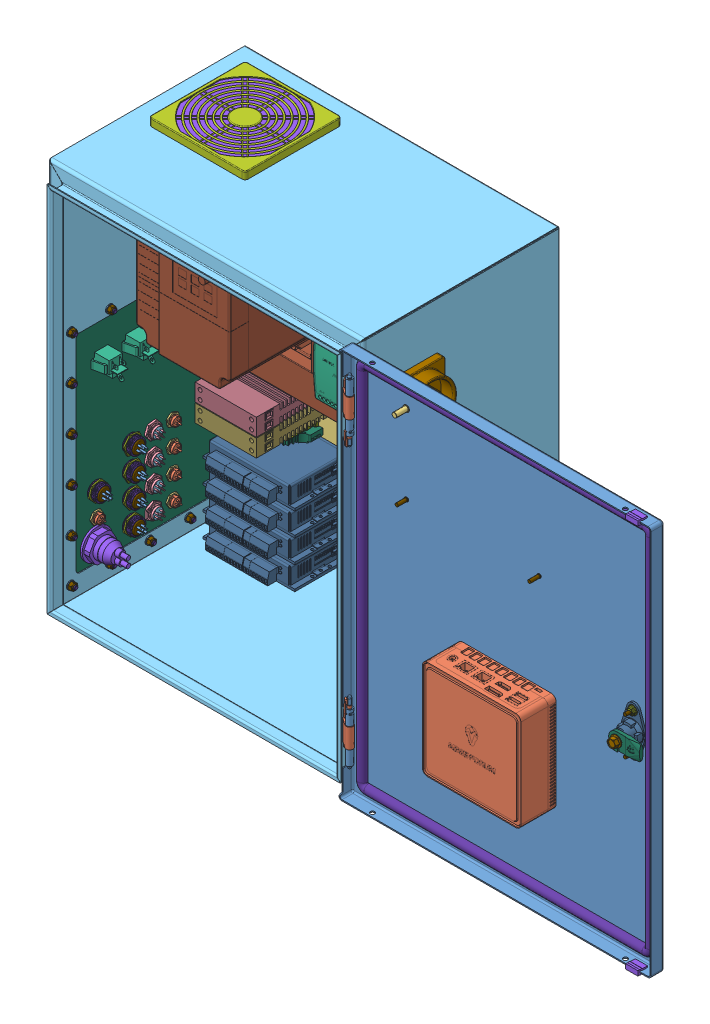
SolidWorks assembly CNC Control Panel, configuration Door Open. Lengths in mm.
Overall size (839.73 526.05 313.88).
272 component instances, 67 part files, 147 mates.
Components (placement in the parent):
- YuCo YC-20X16X10-UL-1: YuCo YC-20X16X10-UL [Door Open] x (-1 0 0) z (0 0 1) size (799.63 509.27 290.8)
  - 87929507-1: 87929507 [Default] at (-197.7898 -139.7 266.2428) x (0 -1 0) z (-0.965926 0 0.258819) size (80.01 7.68 4.83)
    - 87929767-1: 87929767 [Default] at origin size (80.01 4.75 4.75)
    - 87929769_Installed on Pin-1: 87929769_Installed on Pin [Default] at (1.778 3.6068 0) size (17.91 7.45 4.83)
  - 87934540-1: 87934540 [Default] at origin size (406.4 508 269.11)
    - 99401225-1: 99401225 [Default] at (-202.0316 -214.7316 214.7316) x (0 -1 0) z (0 0 1) size (8 16 8)
    - 23271001_After Weld-1: 23271001_After Weld [Default] at (-167.2336 -218.0336 1.1684) x (1 0 0) z (0 -1 0) size (15.88 38.1 15.88)
    - 23271001_After Weld-2: 23271001_After Weld [Default] at (-167.2336 218.0336 1.1684) x (1 0 0) z (0 -1 0) size (15.88 38.1 15.88)
    - 23271001_After Weld-3: 23271001_After Weld [Default] at (167.2336 -218.0336 1.1684) x (1 0 0) z (0 -1 0) size (15.88 38.1 15.88)
    - 23271001_After Weld-4: 23271001_After Weld [Default] at (167.2336 218.0336 1.1684) x (-1 0 0) z (0 1 0) size (15.88 38.1 15.88)
    - 87934343_default-1: 87934343_default [Default] at origin size (406.4 508 269.11)
  - 89076399-1: 89076399 [Default] at (-185.1152 184.15 251.2568) x (0 1 0) z (-1 0 0) size (53.98 24.05 15.83)
    - 89076193-1: 89076193 [Default] at origin size (53.98 23 15.83)
    - 89056623-1: 89056623 [Default] at (0 0 7.112) x (-1 0 0) z (0 -1 0) size (49.12 14 1.57)
  - 89076399-2: 89076399 [Default] at (-185.1152 -184.15 251.2568) x (0 1 0) z (-1 0 0) size (53.98 24.05 15.83)
    - 89076193-1: 89076193 [Default] at origin size (53.98 23 15.83)
    - 89056623-1: 89056623 [Default] at (0 0 7.112) x (-1 0 0) z (0 -1 0) size (49.12 14 1.57)
  - 87937923_assy-1: 87937923_assy [Default] at (-395.0843 0 260.0452) x (-1 0 0) z (0 0 -1) size (402.69 509.27 33.01)
    - 64138001-1: 64138001 [Default] at (179.1589 250.7528 -18.99) x (0 0.043619 0.999048) z (1 0 0) size (12.45 6.6 15.75)
    - 64101001-1: 64101001 [Default] at (163.7162 2.0815 -11.0121) size (45.67 63.4 33.01)
      - 87927840_87927840-1: 87927840_87927840 [Default] at (0.5837 -2.0815 -13.7669) x (0 -1 0) z (0 0 -1) size (14 14 15.97)
      - 64201001-1: 64201001 [Default] at (0.5837 -2.0815 11.0121) size (30.48 63.4 19.81)
      - 87541994_Installed Height-1: 87541994_Installed Height [Default] at (0.5837 -2.0815 -0.4393) x (0 -1 0) z (-1 0 0) size (15.37 3.57 15.57)
      - 87541995-1: 87541995 [Default] at (0.5837 -2.0815 0.0901) size (16.26 16.26 1.78)
      - 64210001-1: 64210001 [Default] at (0.5837 -2.0815 8.7261) size (26.42 26.42 4.55)
      - 64202001-1: 64202001 [Default] at (-17.6801 -2.0815 2.3184) x (1 0 0) z (0 -1 0) size (15.88 25.4 15.88)
      - 64203001-1: 64203001 [Default] at (-128.4369 7.7022 -12.7369) size (40.59 20.36 8)
    - 64138001-2: 64138001 [Default] at (179.1589 -251.3798 -18.99) x (0 0.043619 0.999048) z (1 0 0) size (12.45 6.6 15.75)
    - 87932903-1: 87932903 [Default] at (164.2999 23.8125 -6.4503) x (0 -1 0) z (1 0 0) size (11.43 5.65 11.43)
    - 87932903-2: 87932903 [Default] at (164.2999 -23.8125 -6.4503) x (0 -1 0) z (1 0 0) size (11.43 5.65 11.43)
    - 89057561-1: 89057561 [Default] at (-185.8264 0 0) x (1 0 0) z (0 1 0) size (385.34 6.35 486.94)
    - 87937963_weldment-1: 87937963_weldment [Default] at origin size (402.69 503.96 17.74)
      - 87931362_87931362-1: 87931362_87931362 [Default] at (164.2999 23.8125 0) x (-1 0 0) z (0 -1 0) size (5 13.61 5)
      - 87931362_87931362-2: 87931362_87931362 [Default] at (-129.8829 -110.6678 0) x (1 0 0) z (0 1 0) size (5 13.61 5)
      - 87931362_87931362-3: 87931362_87931362 [Default] at (41.0591 -110.6678 0) x (1 0 0) z (0 1 0) size (5 13.61 5)
      - 87937909-1: 87937909 [Default] at origin size (402.69 503.96 17.74)
      - 99401225-1: 99401225 [Default] at (-129.8829 -212.2678 0) x (1 0 0) z (0 1 0) size (8 16 8)
      - 87931362_87931362-4: 87931362_87931362 [Default] at (164.2999 -23.8125 0) x (-1 0 0) z (0 -1 0) size (5 13.61 5)
  - 87543027-1: 87543027 [Default] at (-198.0692 -184.15 254) x (0 -1 0) z (-1 0 0) size (52.83 16.6 16.78)
  - 87929507-2: 87929507 [Default] at (-197.7898 139.7 266.2428) x (0 1 0) z (0.965926 0 -0.258819) size (80.01 7.68 4.83)
    - 87929767-1: 87929767 [Default] at origin size (80.01 4.75 4.75)
    - 87929769_Installed on Pin-1: 87929769_Installed on Pin [Default] at (1.778 3.6068 0) size (17.91 7.45 4.83)
  - 87543027-2: 87543027 [Default] at (-198.0692 184.15 254) x (0 -1 0) z (-1 0 0) size (52.83 16.6 16.78)
  - 64403004-1: 64403004 [Default] at (0 0 23.5204) size (360.68 462.28 2.46)
- SCN-1000-48-1: SCN-1000-48 [Default] at (102.34 60.64 91.9842) x (0 -1 0) z (0 0 1) size (331 68 132)
  - SCN-1000-48 PSU-1: SCN-1000-48 PSU [Default] at origin size (331 68 132)
  - 19155K930_EQUIPMENT COOLING FAN ACCESSORY-1: 19155K930_EQUIPMENT COOLING FAN ACCESSORY [19155K93] at (145.5 34 -35) x (0 -1 0) z (0 0 1) size (57.8 4.4 57.8)
- ALIM MEAN WELL MDR-1: ALIM MEAN WELL MDR [MDR-60-24] at (75.44 73.64 129.4842) x (-1 0 0) z (0 0 1) size (40 90 100.01)
- ALIM MEAN WELL MDR-2: ALIM MEAN WELL MDR [MDR-60-5] at (33.44 73.64 129.4842) x (-1 0 0) z (0 0 1) size (40 90 100.01)
- AXBB-E-1: AXBB-E [Default] at (38.135 -161.215 36.9842) x (-1 0 0) z (0 1 0) size (97.39 26.5 120)
- UCSB-1: UCSB [Default] at (25.6757 -62.365 38.4842) x (-1 0 0) z (0 1 0) size (116.46 15.11 67.7)
- CNCDrive_Parts_Mount-1: CNCDrive_Parts_Mount [Default] at (38.135 -161.215 28.9842) size (93.95 191.55 11)
- CL57Y Stepper Driver-1: CL57Y Stepper Driver [Default] at (-96.34 -223.14 63.8842) x (0 0 1) z (0 1 0) size (89.31 118 24.2)
- 7578K262_SLOTTED WIRE DUCT WITH SNAP-ON COVER-1: 7578K262_SLOTTED WIRE DUCT WITH SNAP-ON COVER [4in] at (-12.0928 118.3376 25.9842) x (-1 0 0) z (0 1 0) size (39.88 59.94 101.6)
- 8961K150_DIN RAIL (1)-1: 8961K150_DIN RAIL (1) [3.5in] at (510.44 73.64 25.9842) x (0 0 1) z (-1 0 0) size (7.5 35 88.9)
- 7578K262_SLOTTED WIRE DUCT WITH SNAP-ON COVER-3: 7578K262_SLOTTED WIRE DUCT WITH SNAP-ON COVER [10in] at (-158.56 -3.2012 25.9842) x (0 -1 0) z (-1 0 0) size (39.88 59.94 254.14)
- 8961K150_DIN RAIL (1)-2: 8961K150_DIN RAIL (1) [3in] at (-102.84 395.86 25.9842) x (0 0 1) z (0 -1 0) size (7.5 35 76.2)
- 8961K150_DIN RAIL (1)-3: 8961K150_DIN RAIL (1) [5in] at (468.34 183.64 25.9842) x (0 0 1) z (-1 0 0) size (7.5 35 127)
- Lovato Electric FB01F1P-4: Lovato Electric FB01F1P [Default] at (-30.16 183.5289 27.4842) size (17.5 88.8 63.77)
- Lovato Electric FB01F1P-5: Lovato Electric FB01F1P [Default] at (-12.16 183.5289 27.4842) size (17.5 88.8 63.77)
- 7641K526_MODULAR DIN RAIL-MOUNT TERMINAL BLOCK-2: 7641K526_MODULAR DIN RAIL-MOUNT TERMINAL BLOCK [7641K526] at (9.84 186.09 73.9842) x (1 0 0) z (0 -1 0) size (8.38 46.95 44.65)
- 7641K350_MODULAR DIN RAIL-MOUNT TERMINAL BLOCK-1: 7641K350_MODULAR DIN RAIL-MOUNT TERMINAL BLOCK [Default] at (92.64 183.44 27.0092) x (1 0 0) z (0 -1 0) size (10.03 34.98 53.45)
- 7641K924_MODULAR DIN RAIL-MOUNT TERMINAL BLOCK-1: 7641K924_MODULAR DIN RAIL-MOUNT TERMINAL BLOCK [7641K924] at (-105.067 -81.644 73.9842) x (0 1 0) z (1 0 0) size (7 46.95 44.65)
- 7641K350_MODULAR DIN RAIL-MOUNT TERMINAL BLOCK-2: 7641K350_MODULAR DIN RAIL-MOUNT TERMINAL BLOCK [Default] at (-102.64 -101.944 27.0092) x (0 -1 0) z (-1 0 0) size (10.03 34.98 53.45)
- M5 Bolt Nut Washer Assembly-1: M5 Bolt Nut Washer Assembly [Default] at (127.6278 68.7129 256.9715) size (14.92 12.73 12.73) (flexible)
  - Trimcraft M5 BSC-1: Trimcraft M5 BSC [5mm x 12mm SST BSC] at (-336.6778 -21.2987 -233.3857) x (0 0 1) z (-1 0 0) size (9.5 9.5 14.92)
  - Trimcraft M5 Nylock Nut-1: Trimcraft M5 Nylock Nut [M5 Nylock Nut] at (-328.5594 -21.2987 -233.3857) x (0 0 1) z (0 1 0) size (8 5.15 9.24)
  - Trimcraft M5 Washer-1: Trimcraft M5 Washer [M5 Flat Washer] at (-328.5594 -21.2987 -233.3857) x (0 0.07132 0.997453) z (-1 0 0) size (10 10 1.1)
  - Trimcraft M5 Washer-2: Trimcraft M5 Washer [M5 Flat Washer] at (-332.8278 -21.2987 -233.3857) x (0 -0.944717 -0.327887) z (-1 0 0) size (10 10 1.1)
- M5 Bolt Nut Washer Assembly-2: M5 Bolt Nut Washer Assembly [Default] at (129.63 85.8442 76.3307) x (0.969846 0.17101 -0.173648) z (0.198566 -0.141314 0.969846) size (17.7 13.8 13.81) (flexible)
  - Trimcraft M5 BSC-1: Trimcraft M5 BSC [5mm x 12mm SST BSC] at (-334.5346 10.5606 -64.1628) x (-0.198566 0.014245 0.979984) z (-0.969846 0.141314 -0.198566) size (9.5 9.5 14.92)
  - Trimcraft M5 Nylock Nut-1: Trimcraft M5 Nylock Nut [M5 Nylock Nut] at (-326.661 9.4134 -62.5507) x (-0.198566 0.014245 0.979984) z (0.141314 0.989862 0.014245) size (8 5.15 9.24)
  - Trimcraft M5 Washer-1: Trimcraft M5 Washer [M5 Flat Washer] at (-326.661 9.4134 -62.5507) x (-0.187981 0.084806 0.978504) z (-0.969846 0.141314 -0.198566) size (10 10 1.1)
  - Trimcraft M5 Washer-2: Trimcraft M5 Washer [M5 Flat Washer] at (-330.8007 10.0166 -63.3983) x (-0.223661 -0.839732 0.494799) z (-0.969846 0.141314 -0.198566) size (10 10 1.1)
- M5 Bolt Nut Washer Assembly-3: M5 Bolt Nut Washer Assembly [Default] at (129.3262 128.9032 16.2035) x (0.883022 0.321394 -0.34202) z (0.418989 -0.211471 0.883022) size (19.17 14.18 15.7) (flexible)
  - Trimcraft M5 BSC-1: Trimcraft M5 BSC [5mm x 12mm SST BSC] at (-362.0061 31.847 -28.5976) x (-0.418989 0.047054 0.906771) z (-0.883022 0.211471 -0.418989) size (9.5 9.5 14.92)
  - Trimcraft M5 Nylock Nut-1: Trimcraft M5 Nylock Nut [M5 Nylock Nut] at (-354.8374 30.1302 -25.1961) x (-0.418989 0.047054 0.906771) z (0.211471 0.976251 0.047054) size (8 5.15 9.24)
  - Trimcraft M5 Washer-1: Trimcraft M5 Washer [M5 Flat Washer] at (-354.8374 30.1302 -25.1961) x (-0.40284 0.116561 0.907818) z (-0.883022 0.211471 -0.418989) size (10 10 1.1)
  - Trimcraft M5 Washer-2: Trimcraft M5 Washer [M5 Flat Washer] at (-358.6065 31.0329 -26.9845) x (-0.397734 -0.81111 0.428846) z (-0.883022 0.211471 -0.418989) size (10 10 1.1)
- M5 Bolt Nut Washer Assembly-4: M5 Bolt Nut Washer Assembly [Default] at (112.6468 166.765 -45.5219) x (0.75 0.433013 -0.5) z (0.625 -0.216506 0.75) size (19.19 14.4 17.44) (flexible)
  - Trimcraft M5 BSC-1: Trimcraft M5 BSC [5mm x 12mm SST BSC] at (-403.4603 61.6518 -9.2057) x (-0.625 0.077324 0.776786) z (-0.75 0.216506 -0.625) size (9.5 9.5 14.92)
  - Trimcraft M5 Nylock Nut-1: Trimcraft M5 Nylock Nut [M5 Nylock Nut] at (-397.3715 59.8941 -4.1317) x (-0.625 0.077324 0.776786) z (0.216506 0.973214 0.077324) size (8 5.15 9.24)
  - Trimcraft M5 Washer-1: Trimcraft M5 Washer [M5 Flat Washer] at (-397.3715 59.8941 -4.1317) x (-0.607967 0.146537 0.780322) z (-0.75 0.216506 -0.625) size (10 10 1.1)
  - Trimcraft M5 Washer-2: Trimcraft M5 Washer [M5 Flat Washer] at (-400.5728 60.8182 -6.7994) x (-0.508622 -0.792851 0.335694) z (-0.75 0.216506 -0.625) size (10 10 1.1)
- M5 Bolt Nut Washer Assembly-5: M5 Bolt Nut Washer Assembly [Default] at (81.8817 192.9931 -105.544) x (0.586824 0.492404 -0.642788) z (0.790379 -0.175893 0.586824) size (17.94 14.06 18.39) (flexible)
  - Trimcraft M5 BSC-1: Trimcraft M5 BSC [5mm x 12mm SST BSC] at (-455.788 90.5376 -9.5391) x (-0.790379 0.08761 0.606321) z (-0.586824 0.175893 -0.790379) size (9.5 9.5 14.92)
  - Trimcraft M5 Nylock Nut-1: Trimcraft M5 Nylock Nut [M5 Nylock Nut] at (-451.0239 89.1096 -3.1224) x (-0.790379 0.08761 0.606321) z (0.175893 0.980503 0.08761) size (8 5.15 9.24)
  - Trimcraft M5 Washer-1: Trimcraft M5 Washer [M5 Flat Washer] at (-451.0239 89.1096 -3.1224) x (-0.775822 0.157317 0.611025) z (-0.586824 0.175893 -0.790379) size (10 10 1.1)
  - Trimcraft M5 Washer-2: Trimcraft M5 Washer [M5 Flat Washer] at (-453.5287 89.8604 -6.4961) x (-0.559424 -0.793767 0.238702) z (-0.586824 0.175893 -0.790379) size (10 10 1.1)
- M5 Bolt Nut Washer Assembly-6: M5 Bolt Nut Washer Assembly [Default] at (42.0554 202.5261 -160.3334) x (0.413176 0.492404 -0.766044) z (0.903335 -0.115201 0.413176) size (16.19 13.98 18.19) (flexible)
  - Trimcraft M5 BSC-1: Trimcraft M5 BSC [5mm x 12mm SST BSC] at (-504.5231 37.339 -42.4506) x (-0.903335 0.073639 0.422567) z (-0.413176 0.115201 -0.903335) size (9.5 9.5 14.92)
  - Trimcraft M5 Nylock Nut-1: Trimcraft M5 Nylock Nut [M5 Nylock Nut] at (-501.1687 36.4037 -35.1169) x (-0.903335 0.073639 0.422567) z (0.115201 0.990609 0.073639) size (8 5.15 9.24)
  - Trimcraft M5 Washer-1: Trimcraft M5 Washer [M5 Flat Washer] at (-501.1687 36.4037 -35.1169) x (-0.892819 0.144102 0.426743) z (-0.413176 0.115201 -0.903335) size (10 10 1.1)
  - Trimcraft M5 Washer-2: Trimcraft M5 Washer [M5 Flat Washer] at (-502.9323 36.8955 -38.9727) x (-0.565922 -0.809644 0.155594) z (-0.413176 0.115201 -0.903335) size (10 10 1.1)
- M5 Bolt Nut Washer Assembly-7: M5 Bolt Nut Washer Assembly [Default] at (0.1494 192.8274 -206.4354) x (0.25 0.433013 -0.866025) z (0.966506 -0.058013 0.25) size (14.6 13.91 17.25) (flexible)
  - Trimcraft M5 BSC-1: Trimcraft M5 BSC [5mm x 12mm SST BSC] at (-539.5682 -32.6411 -78.8416) x (-0.966506 0.044856 0.252692) z (-0.25 0.058013 -0.966506) size (9.5 9.5 14.92)
  - Trimcraft M5 Nylock Nut-1: Trimcraft M5 Nylock Nut [M5 Nylock Nut] at (-537.5386 -33.1121 -70.9951) x (-0.966506 0.044856 0.252692) z (0.058013 0.997308 0.044856) size (8 5.15 9.24)
  - Trimcraft M5 Washer-1: Trimcraft M5 Washer [M5 Flat Washer] at (-537.5386 -33.1121 -70.9951) x (-0.959908 0.11587 0.255248) z (-0.25 0.058013 -0.966506) size (10 10 1.1)
  - Trimcraft M5 Washer-2: Trimcraft M5 Washer [M5 Flat Washer] at (-538.6057 -32.8644 -75.1206) x (-0.549663 -0.830267 0.092343) z (-0.25 0.058013 -0.966506) size (10 10 1.1)
- M5 Bolt Nut Washer Assembly-8: M5 Bolt Nut Washer Assembly [Default] at (-36.1524 164.5811 -240.7794) x (0.116978 0.321394 -0.939693) z (0.992945 -0.019382 0.116978) size (13.83 13.81 16.1) (flexible)
  - Trimcraft M5 BSC-1: Trimcraft M5 BSC [5mm x 12mm SST BSC] at (-552.028 -118.0059 -111.3957) x (-0.992945 0.01723 0.117314) z (-0.116978 0.019382 -0.992945) size (9.5 9.5 14.92)
  - Trimcraft M5 Nylock Nut-1: Trimcraft M5 Nylock Nut [M5 Nylock Nut] at (-551.0783 -118.1633 -103.3346) x (-0.992945 0.01723 0.117314) z (0.019382 0.999664 0.01723) size (8 5.15 9.24)
  - Trimcraft M5 Washer-1: Trimcraft M5 Washer [M5 Flat Washer] at (-551.0783 -118.1633 -103.3346) x (-0.989034 0.088483 0.118244) z (-0.116978 0.019382 -0.992945) size (10 10 1.1)
  - Trimcraft M5 Washer-2: Trimcraft M5 Washer [M5 Flat Washer] at (-551.5776 -118.0806 -107.5729) x (-0.530282 -0.846575 0.045947) z (-0.116978 0.019382 -0.992945) size (10 10 1.1)
- M5 Bolt Nut Washer Assembly-9: M5 Bolt Nut Washer Assembly [Default] at (-59.9382 121.7476 -260.9631) x (0.030154 0.17101 -0.984808) z (0.999542 -0.002598 0.030154) size (13.77 13.74 15.23) (flexible)
  - Trimcraft M5 BSC-1: Trimcraft M5 BSC [5mm x 12mm SST BSC] at (-536.5111 -212.6794 -133.5477) x (-0.999542 0.002521 0.03016) z (-0.030154 0.002598 -0.999542) size (9.5 9.5 14.92)
  - Trimcraft M5 Nylock Nut-1: Trimcraft M5 Nylock Nut [M5 Nylock Nut] at (-536.2663 -212.7005 -125.433) x (-0.999542 0.002521 0.03016) z (0.002598 0.999993 0.002521) size (8 5.15 9.24)
  - Trimcraft M5 Washer-1: Trimcraft M5 Washer [M5 Flat Washer] at (-536.2663 -212.7005 -125.433) x (-0.996811 0.073834 0.030263) z (-0.030154 0.002598 -0.999542) size (10 10 1.1)
  - Trimcraft M5 Washer-2: Trimcraft M5 Washer [M5 Flat Washer] at (-536.395 -212.6894 -129.6995) x (-0.519331 -0.854467 0.013446) z (-0.030154 0.002598 -0.999542) size (10 10 1.1)
- M5 Bolt Nut Washer Assembly-10: M5 Bolt Nut Washer Assembly [Default] at (-66.4389 70.9384 -265.4779) x (0 0 -1) z (1 0 0) size (13.73 13.73 14.92) (flexible)
  - Trimcraft M5 BSC-1: Trimcraft M5 BSC [5mm x 12mm SST BSC] at (-491.8922 -306.3526 -142.6111) x (-1 0 0) z (0 0 -1) size (9.5 9.5 14.92)
  - Trimcraft M5 Nylock Nut-1: Trimcraft M5 Nylock Nut [M5 Nylock Nut] at (-491.8922 -306.3526 -134.4927) x (-1 0 0) z (0 1 0) size (8 5.15 9.24)
  - Trimcraft M5 Washer-1: Trimcraft M5 Washer [M5 Flat Washer] at (-491.8922 -306.3526 -134.4927) x (-0.997453 0.07132 0) z (0 0 -1) size (10 10 1.1)
  - Trimcraft M5 Washer-2: Trimcraft M5 Washer [M5 Flat Washer] at (-491.8922 -306.3526 -138.7611) x (-0.517345 -0.855777 0) z (0 0 -1) size (10 10 1.1)
- M5 Bolt Nut Washer Assembly-11: M5 Bolt Nut Washer Assembly [Default] at (-53.9864 20.2276 -253.8526) x (0.030154 -0.17101 -0.984808) z (0.999542 0.002598 0.030154) size (13.75 13.73 15.23) (flexible)
  - Trimcraft M5 BSC-1: Trimcraft M5 BSC [5mm x 12mm SST BSC] at (-384.1804 -326.3643 -142.6966) x (-0.999542 -0.002521 0.03016) z (-0.030154 -0.002598 -0.999542) size (9.5 9.5 14.92)
  - Trimcraft M5 Nylock Nut-1: Trimcraft M5 Nylock Nut [M5 Nylock Nut] at (-383.9356 -326.3432 -134.5819) x (-0.999542 -0.002521 0.03016) z (-0.002598 0.999993 -0.002521) size (8 5.15 9.24)
  - Trimcraft M5 Washer-1: Trimcraft M5 Washer [M5 Flat Washer] at (-383.9356 -326.3432 -134.5819) x (-0.997182 0.068806 0.029904) z (-0.030154 -0.002598 -0.999542) size (10 10 1.1)
  - Trimcraft M5 Washer-2: Trimcraft M5 Washer [M5 Flat Washer] at (-384.0643 -326.3543 -138.8484) x (-0.514885 -0.857075 0.017761) z (-0.030154 -0.002598 -0.999542) size (10 10 1.1)
- M5 Bolt Nut Washer Assembly-12: M5 Bolt Nut Washer Assembly [Default] at (-24.3434 -22.3488 -226.6961) x (0.116978 -0.321394 -0.939693) z (0.992945 0.019382 0.116978) size (13.7 13.69 16.1) (flexible)
  - Trimcraft M5 BSC-1: Trimcraft M5 BSC [5mm x 12mm SST BSC] at (-283.4267 -318.8867 -146.404) x (-0.992945 -0.01723 0.117314) z (-0.116978 -0.019382 -0.992945) size (9.5 9.5 14.92)
  - Trimcraft M5 Nylock Nut-1: Trimcraft M5 Nylock Nut [M5 Nylock Nut] at (-282.477 -318.7294 -138.3429) x (-0.992945 -0.01723 0.117314) z (-0.019382 0.999664 -0.01723) size (8 5.15 9.24)
  - Trimcraft M5 Washer-1: Trimcraft M5 Washer [M5 Flat Washer] at (-282.477 -318.7294 -138.3429) x (-0.991799 0.05411 0.115787) z (-0.116978 -0.019382 -0.992945) size (10 10 1.1)
  - Trimcraft M5 Washer-2: Trimcraft M5 Washer [M5 Flat Washer] at (-282.9763 -318.8121 -142.5812) x (-0.497108 -0.864403 0.075437) z (-0.116978 -0.019382 -0.992945) size (10 10 1.1)
- M5 Bolt Nut Washer Assembly-13: M5 Bolt Nut Washer Assembly [Default] at (17.6697 -50.2799 -185.638) x (0.25 -0.433013 -0.866025) z (0.966506 0.058013 0.25) size (14.4 13.61 17.25) (flexible)
  - Trimcraft M5 BSC-1: Trimcraft M5 BSC [5mm x 12mm SST BSC] at (-201.1139 -292.6379 -164.9906) x (-0.966506 -0.044856 0.252692) z (-0.25 -0.058013 -0.966506) size (9.5 9.5 14.92)
  - Trimcraft M5 Nylock Nut-1: Trimcraft M5 Nylock Nut [M5 Nylock Nut] at (-199.0843 -292.167 -157.1441) x (-0.966506 -0.044856 0.252692) z (-0.058013 0.997308 -0.044856) size (8 5.15 9.24)
  - Trimcraft M5 Washer-1: Trimcraft M5 Washer [M5 Flat Washer] at (-199.0843 -292.167 -157.1441) x (-0.968183 0.026387 0.24885) z (-0.25 -0.058013 -0.966506) size (10 10 1.1)
  - Trimcraft M5 Washer-2: Trimcraft M5 Washer [M5 Flat Washer] at (-200.1514 -292.4146 -161.2696) x (-0.450371 -0.876679 0.169116) z (-0.25 -0.058013 -0.966506) size (10 10 1.1)
- M5 Bolt Nut Washer Assembly-14: M5 Bolt Nut Washer Assembly [Default] at (65.1631 -59.733 -133.1705) x (0.413176 -0.492404 -0.766044) z (0.903335 0.115201 0.413176) size (15.84 13.48 18.19) (flexible)
  - Trimcraft M5 BSC-1: Trimcraft M5 BSC [5mm x 12mm SST BSC] at (-146.8744 -260.3388 -203.177) x (-0.903335 -0.073639 0.422567) z (-0.413176 -0.115201 -0.903335) size (9.5 9.5 14.92)
  - Trimcraft M5 Nylock Nut-1: Trimcraft M5 Nylock Nut [M5 Nylock Nut] at (-143.5201 -259.4035 -195.8434) x (-0.903335 -0.073639 0.422567) z (-0.115201 0.990609 -0.073639) size (8 5.15 9.24)
  - Trimcraft M5 Washer-1: Trimcraft M5 Washer [M5 Flat Washer] at (-143.5201 -259.4035 -195.8434) x (-0.909251 -0.002801 0.416239) z (-0.413176 -0.115201 -0.903335) size (10 10 1.1)
  - Trimcraft M5 Washer-2: Trimcraft M5 Washer [M5 Flat Washer] at (-145.2837 -259.8952 -199.6992) x (-0.36875 -0.885837 0.281631) z (-0.413176 -0.115201 -0.903335) size (10 10 1.1)
- M5 Bolt Nut Washer Assembly-15: M5 Bolt Nut Washer Assembly [Default] at (110.5536 -50.1313 -72.4119) x (0.586824 -0.492404 -0.642788) z (0.790379 0.175893 0.586824) size (17.94 13.77 18.39) (flexible)
  - Trimcraft M5 BSC-1: Trimcraft M5 BSC [5mm x 12mm SST BSC] at (-185.3267 -213.2164 -219.3203) x (-0.790379 -0.08761 0.606321) z (-0.586824 -0.175893 -0.790379) size (9.5 9.5 14.92)
  - Trimcraft M5 Nylock Nut-1: Trimcraft M5 Nylock Nut [M5 Nylock Nut] at (-180.5627 -211.7885 -212.9037) x (-0.790379 -0.08761 0.606321) z (-0.175893 0.980503 -0.08761) size (8 5.15 9.24)
  - Trimcraft M5 Washer-1: Trimcraft M5 Washer [M5 Flat Washer] at (-180.5627 -211.7885 -212.9037) x (-0.800911 -0.017457 0.598529) z (-0.586824 -0.175893 -0.790379) size (10 10 1.1)
  - Trimcraft M5 Washer-2: Trimcraft M5 Washer [M5 Flat Washer] at (-183.0675 -212.5392 -216.2773) x (-0.258374 -0.884417 0.388652) z (-0.586824 -0.175893 -0.790379) size (10 10 1.1)
- M5 Bolt Nut Washer Assembly-16: M5 Bolt Nut Washer Assembly [Default] at (147.0168 -24.0539 -6.8171) x (0.75 -0.433013 -0.5) z (0.625 0.216506 0.75) size (19.19 14.14 17.44) (flexible)
  - Trimcraft M5 BSC-1: Trimcraft M5 BSC [5mm x 12mm SST BSC] at (-239.3735 -176.0547 -221.4715) x (-0.625 -0.077324 0.776786) z (-0.75 -0.216506 -0.625) size (9.5 9.5 14.92)
  - Trimcraft M5 Nylock Nut-1: Trimcraft M5 Nylock Nut [M5 Nylock Nut] at (-233.2847 -174.297 -216.3975) x (-0.625 -0.077324 0.776786) z (-0.216506 0.973214 -0.077324) size (8 5.15 9.24)
  - Trimcraft M5 Washer-1: Trimcraft M5 Washer [M5 Flat Washer] at (-233.2847 -174.297 -216.3975) x (-0.63885 -0.007717 0.769293) z (-0.75 -0.216506 -0.625) size (10 10 1.1)
  - Trimcraft M5 Washer-2: Trimcraft M5 Washer [M5 Flat Washer] at (-236.486 -175.2212 -219.0652) x (-0.138059 -0.872857 0.468038) z (-0.75 -0.216506 -0.625) size (10 10 1.1)
- M5 Bolt Nut Washer Assembly-17: M5 Bolt Nut Washer Assembly [Default] at (169.699 13.4874 60.1326) x (0.883022 -0.321394 -0.34202) z (0.418989 0.211471 0.883022) size (19.17 14.02 15.86) (flexible)
  - Trimcraft M5 BSC-1: Trimcraft M5 BSC [5mm x 12mm SST BSC] at (-296.3255 -141.1602 -208.2053) x (-0.418989 -0.047054 0.906771) z (-0.883022 -0.211471 -0.418989) size (9.5 9.5 14.92)
  - Trimcraft M5 Nylock Nut-1: Trimcraft M5 Nylock Nut [M5 Nylock Nut] at (-289.1567 -139.4434 -204.8037) x (-0.418989 -0.047054 0.906771) z (-0.211471 0.976251 -0.047054) size (8 5.15 9.24)
  - Trimcraft M5 Washer-1: Trimcraft M5 Washer [M5 Flat Washer] at (-289.1567 -139.4434 -204.8037) x (-0.433004 0.022692 0.901106) z (-0.883022 -0.211471 -0.418989) size (10 10 1.1)
  - Trimcraft M5 Washer-2: Trimcraft M5 Washer [M5 Flat Washer] at (-292.9258 -140.3461 -206.5921) x (-0.03579 -0.859796 0.509381) z (-0.883022 -0.211471 -0.418989) size (10 10 1.1)
- M5 Bolt Nut Washer Assembly-18: M5 Bolt Nut Washer Assembly [Default] at (176.4401 56.199 125.2253) x (0.969846 -0.17101 -0.173648) z (0.198566 0.141314 0.969846) size (17.7 13.7 13.86) (flexible)
  - Trimcraft M5 BSC-1: Trimcraft M5 BSC [5mm x 12mm SST BSC] at (-344.9995 -100.3732 -184.8732) x (-0.198566 -0.014245 0.979984) z (-0.969846 -0.141314 -0.198566) size (9.5 9.5 14.92)
  - Trimcraft M5 Nylock Nut-1: Trimcraft M5 Nylock Nut [M5 Nylock Nut] at (-337.1259 -99.2259 -183.2612) x (-0.198566 -0.014245 0.979984) z (-0.141314 0.989862 -0.014245) size (8 5.15 9.24)
  - Trimcraft M5 Washer-1: Trimcraft M5 Washer [M5 Flat Washer] at (-337.1259 -99.2259 -183.2612) x (-0.208139 0.056389 0.976473) z (-0.969846 -0.141314 -0.198566) size (10 10 1.1)
  - Trimcraft M5 Washer-2: Trimcraft M5 Washer [M5 Flat Washer] at (-341.2655 -99.8291 -184.1088) x (0.018207 -0.854471 0.51918) z (-0.969846 -0.141314 -0.198566) size (10 10 1.1)
- MinixForum_UM300-1: MinixForum_UM300 [Default] at (402.7142 -68.0148 262.6308) x (1 0 0) z (0 -1 0) size (127 51.25 127.5)
- Power Brick Mount-1: Power Brick Mount [Default] at (107.8566 247.8316 186.1466) x (1 0 0) z (0 -1 0) size (122.03 57.15 18.36)
- UM300 Power Brick-1: UM300 Power Brick [Default] at (107.8566 247.8316 186.1466) x (1 0 0) z (0 1 0) size (114.52 49.52 30)
- 120mm Fan-1: 120mm Fan [Default] at (183.6977 -179 160) x (0 1 0) z (0 0 1) size (121.23 43.53 120.37)
- 120mm Filter-1: 120mm Filter [Default] at (203.2 -179 160) x (0 0 -1) z (1 0 0) size (124.5 124.5 9.5)
  - Base-1: Base [Default] at origin size (120.7 120.7 4.5)
  - Cover-1: Cover [Default] at origin size (124.5 124.5 9.5)
  - Filter Pad-1: Filter Pad [Default] at (0 0 8.5) x (-1 0 0) z (0 0 -1) size (121 121 1)
- 120mm Filter-2: 120mm Filter [Default] at (-113.2 254 90) x (0 0 1) z (0 1 0) size (124.5 124.5 9.5)
  - Base-1: Base [Default] at origin size (120.7 120.7 4.5)
  - Cover-1: Cover [Default] at origin size (124.5 124.5 9.5)
  - Filter Pad-1: Filter Pad [Default] at (0 0 8.5) x (-1 0 0) z (0 0 -1) size (121 121 1)
- ALLEN-BRADLEY_194E-E25-1753-6N-1: ALLEN-BRADLEY_194E-E25-1753-6N [Default] at (139.39 158.492 190) x (0 0 -1) z (1 0 0) size (67.07 77.22 97.54)
- YW1B-V4E11R EMERGENCY STOP (IDEC)-1: YW1B-V4E11R EMERGENCY STOP (IDEC) [Default] at (182.9762 86.3125 146.2923) x (0 1 0) z (1 0 0) size (60.25 60.25 78.3)
  - YW1B-V4E02R EMERGENCY STOP  (IDEC)-1-1: YW1B-V4E02R EMERGENCY STOP  (IDEC)-1 [Default] at (-27.3125 43.7077 20.7238) x (-0.265481 0.964116 0) z (0 0 1) size (28.8 28.8 5)
  - YW1B-V4E02R EMERGENCY STOP  (IDEC)-4-1: YW1B-V4E02R EMERGENCY STOP  (IDEC)-4 [Default] at (-27.3125 33.7077 -2.4762) x (0 1 0) z (0 0 1) size (10 41.4 26.3)
  - YW1B-V4E02R EMERGENCY STOP  (IDEC)-2-1: YW1B-V4E02R EMERGENCY STOP  (IDEC)-2 [Default] at (-27.3125 43.7077 0.9238) x (1 0 0) z (0 -1 0) size (35.5 17.3 30)
  - YW1B-V4E02R EMERGENCY STOP  (IDEC)-3-1: YW1B-V4E02R EMERGENCY STOP  (IDEC)-3 [Default] at (-27.3125 43.7077 9.8238) x (-0.056052 0.998428 0) z (-0.998428 -0.056052 0) size (25.4 5 41.2)
  - YW1B-V4E02R EMERGENCY STOP  (IDEC)-5-1: YW1B-V4E02R EMERGENCY STOP  (IDEC)-5 [Default] at (-27.3125 43.7077 21.5238) size (60.25 60.25 55.5)
  - YW1B-V4E02R EMERGENCY STOP  (IDEC)-4-2: YW1B-V4E02R EMERGENCY STOP  (IDEC)-4 [Default] at (-27.3125 53.7077 -2.4762) x (0 1 0) z (0 0 1) size (10 41.4 26.3)
- Gland Plate Assembly-1: Gland Plate Assembly [Default] at (-203.2 -94 125) x (0 0 1) z (-1 0 0) size (220 318.54 82.81) (flexible)
  - Controller Gland Plate-1: Controller Gland Plate [Default] at origin size (220 300 2)
  - GX20_Aviation_Connector-1: GX20_Aviation_Connector [Bulkhead Only] at (23 -112 -3.5797) x (0.707107 -0.707107 0) z (0 0 -1) size (24.33 25.09 32.91)
    - Female-1: Female [Default] at origin size (24.33 25.09 32.91)
      - nut-1: nut [Default] at origin size (24.33 25.09 4.78)
      - upper sheath-1: upper sheath [Default] at origin size (22.55 22.55 24.17)
      - Inner plastic-1: Inner plastic [Default] at origin size (16.26 16.26 13.66)
      - needle-1: needle [Default] at origin size (2.5 2.57 30.01)
      - needle-2: needle [Default] x (0 1 0) z (0 0 1) size (2.5 2.57 30.01)
      - needle-3: needle [Default] x (-1 0 0) z (0 0 1) size (2.5 2.57 30.01)
      - needle-4: needle [Default] x (0 -1 0) z (0 0 1) size (2.5 2.57 30.01)
  - GX20_Aviation_Connector-2: GX20_Aviation_Connector [Bulkhead Only] at (23 -82 -3.5797) x (0.810276 -0.586049 0) z (0 0 -1) size (24.33 25.09 32.91)
    - Female-1: Female [Default] at origin size (24.33 25.09 32.91)
      - nut-1: nut [Default] at origin size (24.33 25.09 4.78)
      - upper sheath-1: upper sheath [Default] at origin size (22.55 22.55 24.17)
      - Inner plastic-1: Inner plastic [Default] at origin size (16.26 16.26 13.66)
      - needle-1: needle [Default] at origin size (2.5 2.57 30.01)
      - needle-2: needle [Default] x (0 1 0) z (0 0 1) size (2.5 2.57 30.01)
      - needle-3: needle [Default] x (-1 0 0) z (0 0 1) size (2.5 2.57 30.01)
      - needle-4: needle [Default] x (0 -1 0) z (0 0 1) size (2.5 2.57 30.01)
  - GX20_Aviation_Connector-3: GX20_Aviation_Connector [Bulkhead Only] at (23 -52 -3.5797) x (0.878303 -0.478104 0) z (0 0 -1) size (24.33 25.09 32.91)
    - Female-1: Female [Default] at origin size (24.33 25.09 32.91)
      - nut-1: nut [Default] at origin size (24.33 25.09 4.78)
      - upper sheath-1: upper sheath [Default] at origin size (22.55 22.55 24.17)
      - Inner plastic-1: Inner plastic [Default] at origin size (16.26 16.26 13.66)
      - needle-1: needle [Default] at origin size (2.5 2.57 30.01)
      - needle-2: needle [Default] x (0 1 0) z (0 0 1) size (2.5 2.57 30.01)
      - needle-3: needle [Default] x (-1 0 0) z (0 0 1) size (2.5 2.57 30.01)
      - needle-4: needle [Default] x (0 -1 0) z (0 0 1) size (2.5 2.57 30.01)
  - GX20_Aviation_Connector-4: GX20_Aviation_Connector [Bulkhead Only] at (23 -22 -3.5797) x (0.919044 -0.394154 0) z (0 0 -1) size (24.33 25.09 32.91)
    - Female-1: Female [Default] at origin size (24.33 25.09 32.91)
      - nut-1: nut [Default] at origin size (24.33 25.09 4.78)
      - upper sheath-1: upper sheath [Default] at origin size (22.55 22.55 24.17)
      - Inner plastic-1: Inner plastic [Default] at origin size (16.26 16.26 13.66)
      - needle-1: needle [Default] at origin size (2.5 2.57 30.01)
      - needle-2: needle [Default] x (0 1 0) z (0 0 1) size (2.5 2.57 30.01)
      - needle-3: needle [Default] x (-1 0 0) z (0 0 1) size (2.5 2.57 30.01)
      - needle-4: needle [Default] x (0 -1 0) z (0 0 1) size (2.5 2.57 30.01)
  - GX12-3P v3-1: GX12-3P v3 [Default] at (-30 -112 2) x (-1 0 0) z (0 1 0) size (16.71 20.71 16.7)
    - GX12-3P-1: GX12-3P [Default] at origin size (14.8 20.71 14.8)
    - Nut M12x0.75 H=1.8mm v2-1: Nut M12x0.75 H=1.8mm v2 [Default] at (0 -4.8 0) x (-1 0 0) z (0 1 0) size (16.71 16.7 2.58)
  - GX12-3P v3-2: GX12-3P v3 [Default] at (-30 -82 2) x (-0.987351 -0.158553 0) z (-0.158553 0.987351 0) size (16.71 20.71 16.7)
    - GX12-3P-1: GX12-3P [Default] at origin size (14.8 20.71 14.8)
    - Nut M12x0.75 H=1.8mm v2-1: Nut M12x0.75 H=1.8mm v2 [Default] at (0 -4.8 0) x (-1 0 0) z (0 1 0) size (16.71 16.7 2.58)
  - GX12-3P v3-3: GX12-3P v3 [Default] at (-30 -52 2) x (-0.959125 -0.282984 0) z (-0.282984 0.959125 0) size (16.71 20.71 16.7)
    - GX12-3P-1: GX12-3P [Default] at origin size (14.8 20.71 14.8)
    - Nut M12x0.75 H=1.8mm v2-1: Nut M12x0.75 H=1.8mm v2 [Default] at (0 -4.8 0) x (-1 0 0) z (0 1 0) size (16.71 16.7 2.58)
  - GX12-3P v3-4: GX12-3P v3 [Default] at (-30 -22 2) x (-0.928571 -0.371154 0) z (-0.371154 0.928571 0) size (16.71 20.71 16.7)
    - GX12-3P-1: GX12-3P [Default] at origin size (14.8 20.71 14.8)
    - Nut M12x0.75 H=1.8mm v2-1: Nut M12x0.75 H=1.8mm v2 [Default] at (0 -4.8 0) x (-1 0 0) z (0 1 0) size (16.71 16.7 2.58)
  - GX16-6-1: GX16-6 [Default] at (-5.5 -112 4) x (0 1 0) z (1 0 0) size (21.98 22.32 21.95)
    - GX16-6-1: GX16-6 [Default] at origin size (21.98 22.32 21.95)
    - Acetal-1: Acetal [Default] at origin size (13 9.8 13)
  - GX16-6-2: GX16-6 [Default] at (-5.5 -82 4) x (-0.158553 0.987351 0) z (0.987351 0.158553 0) size (21.98 22.32 21.95)
    - GX16-6-1: GX16-6 [Default] at origin size (21.98 22.32 21.95)
    - Acetal-1: Acetal [Default] at origin size (13 9.8 13)
  - GX16-6-3: GX16-6 [Default] at (-5.5 -52 4) x (-0.282984 0.959125 0) z (0.959125 0.282984 0) size (21.98 22.32 21.95)
    - GX16-6-1: GX16-6 [Default] at origin size (21.98 22.32 21.95)
    - Acetal-1: Acetal [Default] at origin size (13 9.8 13)
  - GX16-6-4: GX16-6 [Default] at (-5.5 -22 4) x (-0.371154 0.928571 0) z (0.928571 0.371154 0) size (21.98 22.32 21.95)
    - GX16-6-1: GX16-6 [Default] at origin size (21.98 22.32 21.95)
    - Acetal-1: Acetal [Default] at origin size (13 9.8 13)
  - Female US 3 Pin Power Socket Plug Panel Mount-1: Female US 3 Pin Power Socket Plug Panel Mount [Default] at (60 90.075 2) size (28.15 27.25 33.25)
  - Female US 3 Pin Power Socket Plug Panel Mount-2: Female US 3 Pin Power Socket Plug Panel Mount [Default] at (20 90.075 2) size (28.15 27.25 33.25)
  - CNLINKO LP24 4pin Connector-1: CNLINKO LP24 4pin Connector [Default] at (-20 90 2) size (33 35.76 36.2)
  - BATIGE USB3_HDMI_Panel_Mount-1: BATIGE USB3_HDMI_Panel_Mount [Default] at (68 -112 9.891) x (0 0 -1) z (1 0 0) size (81.53 75.94 38.8)
  - 7529K191_STRAIGHT CORD GRIP-1: 7529K191_STRAIGHT CORD GRIP [Default] at (-65 90 -11.97) size (35.05 36.66 52.9)
  - GX12-3P v3-5: GX12-3P v3 [Default] at (68 -82 2) x (-1 0 0) z (0 1 0) size (16.71 20.71 16.7)
    - GX12-3P-1: GX12-3P [Default] at origin size (14.8 20.71 14.8)
    - Nut M12x0.75 H=1.8mm v2-1: Nut M12x0.75 H=1.8mm v2 [Default] at (0 -4.8 0) x (-1 0 0) z (0 1 0) size (16.71 16.7 2.58)
  - GX20_Aviation_Connector-5: GX20_Aviation_Connector [Bulkhead Only] at (68 -52 -3.5797) x (0.729168 -0.684335 0) z (0 0 -1) size (24.33 25.09 32.91)
    - Female-1: Female [Default] at origin size (24.33 25.09 32.91)
      - nut-1: nut [Default] at origin size (24.33 25.09 4.78)
      - upper sheath-1: upper sheath [Default] at origin size (22.55 22.55 24.17)
      - Inner plastic-1: Inner plastic [Default] at origin size (16.26 16.26 13.66)
      - needle-1: needle [Default] at origin size (2.5 2.57 30.01)
      - needle-2: needle [Default] x (0 1 0) z (0 0 1) size (2.5 2.57 30.01)
      - needle-3: needle [Default] x (-1 0 0) z (0 0 1) size (2.5 2.57 30.01)
      - needle-4: needle [Default] x (0 -1 0) z (0 0 1) size (2.5 2.57 30.01)
- IceSpring_USB3_X2_Panel_Mount-1: IceSpring_USB3_X2_Panel_Mount [Default] at (211.091 -26 190) x (-1 0 0) z (0 0 -1) size (81.53 75.94 38.8)
- GT-2R2G-2 (220V) Huanyang VFD-1: GT-2R2G-2 (220V) Huanyang VFD [Default] at (-99.5316 125.3316 25.9842) size (125 175 167.8)
- CL57Y Stepper Driver-6: CL57Y Stepper Driver [Default] at (-96.34 -193.14 63.8842) x (0 0 1) z (0 1 0) size (89.31 118 24.2)
